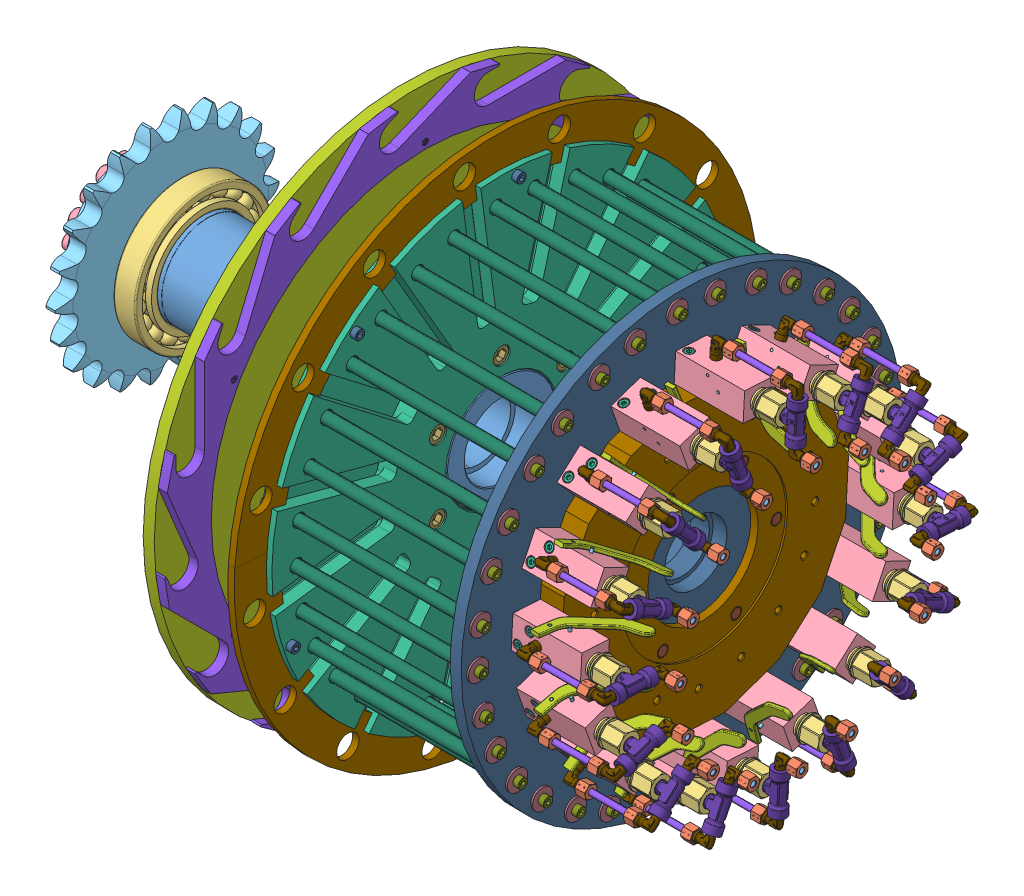
SolidWorks assembly Assieme1, configuration Default. Lengths in mm.
Overall size (749.63 778.63 778.63).
555 component instances, 28 part files, 75 mates.
Components (placement in the parent):
- albero rotazione piatti-1: albero rotazione piatti [Default] at (60.413 18.3637 415) size (415 200 200)
- seger 100mm-1: seger 100mm [KS 1336 E - 100] at (-146.4567 18.3637 415) x (0 0 -1) z (1 0 0) size (107.55 112.98 3)
- SKF - 6020 - 20,DE,NC,20_68-1: SKF - 6020 - 20,DE,NC,20_68 [SKF - 6020 - 20,DE,NC,20_68] at (-131.4567 18.3637 415) x (1 0 0) z (0 -0.434476 -0.900684) size (24 150 150)
- calettatore d95-1: calettatore d95 [Default] at (-184.9572 18.3637 415) size (39.5 135 135)
- pulegia z =50-1: pulegia z =50 [Chain wheel ISO - 22Z 20A-1 --22SB150H40L95.0N] at (-173.9167 18.3637 415) size (40 241.57 243.73)
- Disco supporto montaggio e Colonne-1: Disco supporto montaggio e Colonne [Default] at (204.0433 18.3637 415) x (0 -0.866025 -0.5) z (1 0 0) size (499.6 499.6 29)
- SKF - 6020 - 20,DE,NC,20_68-2: SKF - 6020 - 20,DE,NC,20_68 [SKF - 6020 - 20,DE,NC,20_68] at (62.0433 18.3637 415) x (1 0 0) z (0 -0.432628 -0.901573) size (24 150 150)
- piatto rotante porta tappi-1: piatto rotante porta tappi [Default] at (99.0433 18.3637 415) x (0 0 -1) z (1 0 0) size (570 570 20.57)
- disco trasportatore tappi 31-1: disco trasportatore tappi 31 [Default] at (111.0433 18.3637 415) x (0 0.5 -0.866025) z (1 0 0) size (570 570 10.42)
- Distributore Rotante-1: Distributore Rotante [Default] at (425.0433 18.3637 415) x (0 -0.055301 -0.99847) z (1 0 0) size (310 310 25.54)
- disco trascinato porta distributore vuoto-1: disco trascinato porta distributore vuoto [Default] at (400.0433 18.3637 415) x (0 0.055301 0.99847) z (-1 0 0) size (480 480 50)
- m12 35mm-1: m12 35mm [ISO 4762 M12 x 35 - 35N] at (376.0433 -53.0243 378.8925) x (1 0 0) z (0 -0.5 0.866025) size (47 18 18)
- m12 90mm-3: m12 90mm [ISO 4762 M12 x 90 - 90N] at (203.0433 -21.6363 345.718) x (-1 0 0) z (0 -0.5 0.866025) size (102 18 18)
- rondella m6 22mm-1: rondella m6 22mm [Washer ISO 7094 - 6] at (99.0433 -101.6363 207.1539) x (1 0 0) z (0 -1 0) size (2 22 22)
- M6 20mm-1: M6 20mm [ISO 4762 M6 x 20 - 20N] at (91.0433 -101.6363 207.1539) x (1 0 0) z (0 0.5 0.866025) size (26 10 10)
- m12 35mm-2: m12 35mm [ISO 4762 M12 x 35 - 35N] at (376.0433 13.9397 335.1224) x (1 0 0) z (0 -1 0) size (47 18 18)
- m12 35mm-3: m12 35mm [ISO 4762 M12 x 35 - 35N] at (376.0433 85.3277 371.2299) x (1 0 0) z (0 -0.5 -0.866025) size (47 18 18)
- m12 35mm-4: m12 35mm [ISO 4762 M12 x 35 - 35N] at (376.0433 89.7517 451.1075) x (1 0 0) z (0 0.5 -0.866025) size (47 18 18)
- m12 35mm-5: m12 35mm [ISO 4762 M12 x 35 - 35N] at (376.0433 22.7877 494.8776) x (1 0 0) z (0 1 0) size (47 18 18)
- m12 35mm-6: m12 35mm [ISO 4762 M12 x 35 - 35N] at (376.0433 -48.6003 458.7701) x (1 0 0) z (0 0.5 0.866025) size (47 18 18)
- rondella m6 22mm-2: rondella m6 22mm [Washer ISO 7094 - 6] at (99.0433 138.3637 207.1539) x (1 0 0) z (0 -0.5 -0.866025) size (2 22 22)
- rondella m6 22mm-3: rondella m6 22mm [Washer ISO 7094 - 6] at (99.0433 258.3637 415) x (1 0 0) z (0 0.5 -0.866025) size (2 22 22)
- rondella m6 22mm-4: rondella m6 22mm [Washer ISO 7094 - 6] at (99.0433 138.3637 622.8461) x (1 0 0) z (0 1 0) size (2 22 22)
- rondella m6 22mm-5: rondella m6 22mm [Washer ISO 7094 - 6] at (99.0433 -101.6363 622.8461) x (1 0 0) z (0 0.5 0.866025) size (2 22 22)
- rondella m6 22mm-6: rondella m6 22mm [Washer ISO 7094 - 6] at (99.0433 -221.6363 415) x (1 0 0) z (0 -0.5 0.866025) size (2 22 22)
- M6 20mm-2: M6 20mm [ISO 4762 M6 x 20 - 20N] at (91.0433 138.3637 207.1539) x (1 0 0) z (0 -0.5 0.866025) size (26 10 10)
- M6 20mm-3: M6 20mm [ISO 4762 M6 x 20 - 20N] at (91.0433 258.3637 415) x (1 0 0) z (0 -1 0) size (26 10 10)
- M6 20mm-4: M6 20mm [ISO 4762 M6 x 20 - 20N] at (91.0433 138.3637 622.8461) x (1 0 0) z (0 -0.5 -0.866025) size (26 10 10)
- M6 20mm-5: M6 20mm [ISO 4762 M6 x 20 - 20N] at (91.0433 -101.6363 622.8461) x (1 0 0) z (0 0.5 -0.866025) size (26 10 10)
- M6 20mm-6: M6 20mm [ISO 4762 M6 x 20 - 20N] at (91.0433 -221.6363 415) x (1 0 0) z (0 1 0) size (26 10 10)
- m12 90mm-4: m12 90mm [ISO 4762 M12 x 90 - 90N] at (203.0433 58.3637 345.718) x (-1 0 0) z (0 -1 0) size (102 18 18)
- m12 90mm-5: m12 90mm [ISO 4762 M12 x 90 - 90N] at (203.0433 98.3637 415) x (-1 0 0) z (0 -0.5 -0.866025) size (102 18 18)
- m12 90mm-6: m12 90mm [ISO 4762 M12 x 90 - 90N] at (203.0433 58.3637 484.282) x (-1 0 0) z (0 0.5 -0.866025) size (102 18 18)
- m12 90mm-7: m12 90mm [ISO 4762 M12 x 90 - 90N] at (203.0433 -21.6363 484.282) x (-1 0 0) z (0 1 0) size (102 18 18)
- m12 90mm-8: m12 90mm [ISO 4762 M12 x 90 - 90N] at (203.0433 -61.6363 415) x (-1 0 0) z (0 0.5 0.866025) size (102 18 18)
- asta scorrimento carello-1: asta scorrimento carello [Default] at (287.5433 70.1437 197.9013) x (0 0 -1) z (1 0 0) size (12 12 225)
- rondella m6 22mm-7: rondella m6 22mm [Washer ISO 7094 - 6] at (175.0433 70.1437 197.9013) x (1 0 0) z (0 -1 0) size (2 22 22)
- M6 16mm-1: M6 16mm [ISO 4762 M6 x 16 - 16N] at (167.0433 70.1437 197.9013) size (22 10 10)
- M6 16mm-2: M6 16mm [ISO 4762 M6 x 16 - 16N] at (408.0433 70.1437 197.9013) x (-1 0 0) z (0 0 -1) size (22 10 10)
- rondella m6 22mm-8: rondella m6 22mm [Washer ISO 7094 - 6] at (400.0433 70.1437 197.9013) x (-1 0 0) z (0 1 0) size (2 22 22)
- rondella m6 22mm-9: rondella m6 22mm [Washer ISO 7094 - 6] at (175.0433 24.5373 191.8971) x (1 0 0) z (0 -0.965926 -0.258819) size (2 22 22)
- M6 16mm-3: M6 16mm [ISO 4762 M6 x 16 - 16N] at (167.0433 24.5373 191.8971) x (1 0 0) z (0 0.258819 -0.965926) size (22 10 10)
- asta scorrimento carello-2: asta scorrimento carello [Default] at (287.5433 24.5373 191.8971) x (0 0.258819 -0.965926) z (-1 0 0) size (12 12 225)
- rondella m6 22mm-10: rondella m6 22mm [Washer ISO 7094 - 6] at (400.0433 24.5373 191.8971) x (-1 0 0) z (0 0.965926 0.258819) size (2 22 22)
- M6 16mm-4: M6 16mm [ISO 4762 M6 x 16 - 16N] at (408.0433 24.5373 191.8971) x (-1 0 0) z (0 -0.258819 0.965926) size (22 10 10)
- AssiemeValvola-1: AssiemeValvola [Default] at (515.3257 74.6348 254.5832) x (0 -0.331007 0.943628) z (0 0.943628 0.331007) size (90.26 138.63 38)
  - RaccordoT-1: RaccordoT [Default] at origin size (43 29.75 16.5)
  - Raccordo a L-1: Raccordo a L [Default] at (-30 0 0) x (0 -1 0) z (0 0 -1) size (28.34 25.51 14.01)
    - 1809_06_10_01-1: 1809_06_10_01 [Default] at origin size (22.49 23 10)
    - 1809_06_10_02-1: 1809_06_10_02 [Default] at origin size (6.5 8.5 8.5)
    - 1809_06_10_03-1: 1809_06_10_03 [Default] at origin size (11.02 15.01 14.01)
  - Raccordo a L-2: Raccordo a L [Default] at (30 0 0) x (0 1 0) z (0 0 -1) size (28.34 25.51 14.01)
    - 1809_06_10_01-1: 1809_06_10_01 [Default] at origin size (22.49 23 10)
    - 1809_06_10_02-1: 1809_06_10_02 [Default] at origin size (6.5 8.5 8.5)
    - 1809_06_10_03-1: 1809_06_10_03 [Default] at origin size (11.02 15.01 14.01)
  - TappoChiusura-1: TappoChiusura [Default] at (0 -32 0) x (0 -1 0) z (0 0 1) size (38.28 26.74 26.74)
  - CorpoValvola-1: CorpoValvola [Default] at (-15 -115.2824 0) size (30 75 34)
  - Raccordo a L-3: Raccordo a L [Default] at (-30 -88.2824 0) x (0 1 0) z (0 0 1) size (28.34 25.51 14.01)
    - 1809_06_10_01-1: 1809_06_10_01 [Default] at origin size (22.49 23 10)
    - 1809_06_10_02-1: 1809_06_10_02 [Default] at origin size (6.5 8.5 8.5)
    - 1809_06_10_03-1: 1809_06_10_03 [Default] at origin size (11.02 15.01 14.01)
  - Spina_3x38-1: Spina_3x38 [Default] at (0 -68.2824 -21) x (-1 0 0) z (0 0 1) size (3 3 38)
  - Spina_3x38-2: Spina_3x38 [Default] at (-10 -80.2824 -21) x (0.996193 0.087174 0) z (0 0 1) size (3 3 38)
  - M5 40mm-3: M5 40mm [ISO 4762 M5 x 40 - 40N] at (-14.6 -108.7824 9) size (45 8.5 8.5)
  - M5 40mm-2: M5 40mm [ISO 4762 M5 x 40 - 40N] at (-14.6 -96.7824 -9) size (45 8.5 8.5)
  - LevaValvola-1: LevaValvola [Default] at (-24.507 -86.571 -17) x (0.996193 0.087174 0) z (0 0 1) size (77.55 60.2 4)
  - Tubo-1: Tubo [Default] at (-30 -15.9665 0) x (1 0 0) z (0 -1 0) size (6 6 56.4)
- M6 16mm-5: M6 16mm [ISO 4762 M6 x 16 - 16N] at (167.0433 -16.8778 194.6116) x (1 0 0) z (0 0.382683 0.92388) size (22 10 10)
- M6 16mm-6: M6 16mm [ISO 4762 M6 x 16 - 16N] at (167.0433 -98.5342 224.874) x (1 0 0) z (0 0.707107 0.707107) size (22 10 10)
- M6 16mm-7: M6 16mm [ISO 4762 M6 x 16 - 16N] at (167.0433 -162.3939 284.0814) x (1 0 0) z (0 0.92388 0.382683) size (22 10 10)
- M6 16mm-8: M6 16mm [ISO 4762 M6 x 16 - 16N] at (167.0433 -198.735 363.22) x (1 0 0) z (0 1 0) size (22 10 10)
- M6 16mm-9: M6 16mm [ISO 4762 M6 x 16 - 16N] at (167.0433 -202.0247 450.2415) x (1 0 0) z (0 0.92388 -0.382683) size (22 10 10)
- M6 16mm-10: M6 16mm [ISO 4762 M6 x 16 - 16N] at (167.0433 -171.7623 531.8979) x (1 0 0) z (0 0.707107 -0.707107) size (22 10 10)
- M6 16mm-11: M6 16mm [ISO 4762 M6 x 16 - 16N] at (167.0433 -112.5549 595.7576) x (1 0 0) z (0 0.382683 -0.92388) size (22 10 10)
- M6 16mm-12: M6 16mm [ISO 4762 M6 x 16 - 16N] at (167.0433 -33.4163 632.0987) x (1 0 0) z (0 0 -1) size (22 10 10)
- M6 16mm-13: M6 16mm [ISO 4762 M6 x 16 - 16N] at (167.0433 53.6052 635.3884) x (1 0 0) z (0 -0.382683 -0.92388) size (22 10 10)
- M6 16mm-14: M6 16mm [ISO 4762 M6 x 16 - 16N] at (167.0433 135.2616 605.126) x (1 0 0) z (0 -0.707107 -0.707107) size (22 10 10)
- M6 16mm-15: M6 16mm [ISO 4762 M6 x 16 - 16N] at (167.0433 199.1213 545.9186) x (1 0 0) z (0 -0.92388 -0.382683) size (22 10 10)
- M6 16mm-16: M6 16mm [ISO 4762 M6 x 16 - 16N] at (167.0433 235.4624 466.78) x (1 0 0) z (0 -1 0) size (22 10 10)
- M6 16mm-17: M6 16mm [ISO 4762 M6 x 16 - 16N] at (167.0433 238.7521 379.7585) x (1 0 0) z (0 -0.92388 0.382683) size (22 10 10)
- M6 16mm-18: M6 16mm [ISO 4762 M6 x 16 - 16N] at (167.0433 208.4897 298.1021) x (1 0 0) z (0 -0.707107 0.707107) size (22 10 10)
- M6 16mm-19: M6 16mm [ISO 4762 M6 x 16 - 16N] at (167.0433 149.2823 234.2424) x (1 0 0) z (0 -0.382683 0.92388) size (22 10 10)
- rondella m6 22mm-11: rondella m6 22mm [Washer ISO 7094 - 6] at (175.0433 -16.8778 194.6116) x (1 0 0) z (0 -0.92388 0.382683) size (2 22 22)
- rondella m6 22mm-12: rondella m6 22mm [Washer ISO 7094 - 6] at (175.0433 -98.5342 224.874) x (1 0 0) z (0 -0.707107 0.707107) size (2 22 22)
- rondella m6 22mm-13: rondella m6 22mm [Washer ISO 7094 - 6] at (175.0433 -162.3939 284.0814) x (1 0 0) z (0 -0.382683 0.92388) size (2 22 22)
- rondella m6 22mm-14: rondella m6 22mm [Washer ISO 7094 - 6] at (175.0433 -198.735 363.22) size (2 22 22)
- rondella m6 22mm-15: rondella m6 22mm [Washer ISO 7094 - 6] at (175.0433 -202.0247 450.2415) x (1 0 0) z (0 0.382683 0.92388) size (2 22 22)
- rondella m6 22mm-16: rondella m6 22mm [Washer ISO 7094 - 6] at (175.0433 -171.7623 531.8979) x (1 0 0) z (0 0.707107 0.707107) size (2 22 22)
- rondella m6 22mm-17: rondella m6 22mm [Washer ISO 7094 - 6] at (175.0433 -112.5549 595.7576) x (1 0 0) z (0 0.92388 0.382683) size (2 22 22)
- rondella m6 22mm-18: rondella m6 22mm [Washer ISO 7094 - 6] at (175.0433 -33.4163 632.0987) x (1 0 0) z (0 1 0) size (2 22 22)
- rondella m6 22mm-19: rondella m6 22mm [Washer ISO 7094 - 6] at (175.0433 53.6052 635.3884) x (1 0 0) z (0 0.92388 -0.382683) size (2 22 22)
- rondella m6 22mm-20: rondella m6 22mm [Washer ISO 7094 - 6] at (175.0433 135.2616 605.126) x (1 0 0) z (0 0.707107 -0.707107) size (2 22 22)
- rondella m6 22mm-21: rondella m6 22mm [Washer ISO 7094 - 6] at (175.0433 199.1213 545.9186) x (1 0 0) z (0 0.382683 -0.92388) size (2 22 22)
- rondella m6 22mm-22: rondella m6 22mm [Washer ISO 7094 - 6] at (175.0433 235.4624 466.78) x (1 0 0) z (0 0 -1) size (2 22 22)
- rondella m6 22mm-23: rondella m6 22mm [Washer ISO 7094 - 6] at (175.0433 238.7521 379.7585) x (1 0 0) z (0 -0.382683 -0.92388) size (2 22 22)
- rondella m6 22mm-24: rondella m6 22mm [Washer ISO 7094 - 6] at (175.0433 208.4897 298.1021) x (1 0 0) z (0 -0.707107 -0.707107) size (2 22 22)
- rondella m6 22mm-25: rondella m6 22mm [Washer ISO 7094 - 6] at (175.0433 149.2823 234.2424) x (1 0 0) z (0 -0.92388 -0.382683) size (2 22 22)
- asta scorrimento carello-3: asta scorrimento carello [Default] at (287.5433 -16.8778 194.6116) x (0 -0.382683 -0.92388) z (1 0 0) size (12 12 225)
- asta scorrimento carello-4: asta scorrimento carello [Default] at (287.5433 -98.5342 224.874) x (0 -0.707107 -0.707107) z (1 0 0) size (12 12 225)
- asta scorrimento carello-5: asta scorrimento carello [Default] at (287.5433 -162.3939 284.0814) x (0 -0.92388 -0.382683) z (1 0 0) size (12 12 225)
- asta scorrimento carello-6: asta scorrimento carello [Default] at (287.5433 -198.735 363.22) x (0 -1 0) z (1 0 0) size (12 12 225)
- asta scorrimento carello-7: asta scorrimento carello [Default] at (287.5433 -202.0247 450.2415) x (0 -0.92388 0.382683) z (1 0 0) size (12 12 225)
- asta scorrimento carello-8: asta scorrimento carello [Default] at (287.5433 -171.7623 531.8979) x (0 -0.707107 0.707107) z (1 0 0) size (12 12 225)
- asta scorrimento carello-9: asta scorrimento carello [Default] at (287.5433 -112.5549 595.7576) x (0 -0.382683 0.92388) z (1 0 0) size (12 12 225)
- asta scorrimento carello-10: asta scorrimento carello [Default] at (287.5433 -33.4163 632.0987) x (0 0 1) z (1 0 0) size (12 12 225)
- asta scorrimento carello-11: asta scorrimento carello [Default] at (287.5433 53.6052 635.3884) x (0 0.382683 0.92388) z (1 0 0) size (12 12 225)
- asta scorrimento carello-12: asta scorrimento carello [Default] at (287.5433 135.2616 605.126) x (0 0.707107 0.707107) z (1 0 0) size (12 12 225)
- asta scorrimento carello-13: asta scorrimento carello [Default] at (287.5433 199.1213 545.9186) x (0 0.92388 0.382683) z (1 0 0) size (12 12 225)
- asta scorrimento carello-14: asta scorrimento carello [Default] at (287.5433 235.4624 466.78) x (0 1 0) z (1 0 0) size (12 12 225)
- asta scorrimento carello-15: asta scorrimento carello [Default] at (287.5433 238.7521 379.7585) x (0 0.92388 -0.382683) z (1 0 0) size (12 12 225)
- asta scorrimento carello-16: asta scorrimento carello [Default] at (287.5433 208.4897 298.1021) x (0 0.707107 -0.707107) z (1 0 0) size (12 12 225)
- asta scorrimento carello-17: asta scorrimento carello [Default] at (287.5433 149.2823 234.2424) x (0 0.382683 -0.92388) z (1 0 0) size (12 12 225)
- M6 16mm-20: M6 16mm [ISO 4762 M6 x 16 - 16N] at (408.0433 -16.8778 194.6116) x (-1 0 0) z (0 -0.382683 -0.92388) size (22 10 10)
- M6 16mm-21: M6 16mm [ISO 4762 M6 x 16 - 16N] at (408.0433 -98.5342 224.874) x (-1 0 0) z (0 -0.707107 -0.707107) size (22 10 10)
- M6 16mm-22: M6 16mm [ISO 4762 M6 x 16 - 16N] at (408.0433 -162.3939 284.0814) x (-1 0 0) z (0 -0.92388 -0.382683) size (22 10 10)
- M6 16mm-23: M6 16mm [ISO 4762 M6 x 16 - 16N] at (408.0433 -198.735 363.22) x (-1 0 0) z (0 -1 0) size (22 10 10)
- M6 16mm-24: M6 16mm [ISO 4762 M6 x 16 - 16N] at (408.0433 -202.0247 450.2415) x (-1 0 0) z (0 -0.92388 0.382683) size (22 10 10)
- M6 16mm-25: M6 16mm [ISO 4762 M6 x 16 - 16N] at (408.0433 -171.7623 531.8979) x (-1 0 0) z (0 -0.707107 0.707107) size (22 10 10)
- M6 16mm-26: M6 16mm [ISO 4762 M6 x 16 - 16N] at (408.0433 -112.5549 595.7576) x (-1 0 0) z (0 -0.382683 0.92388) size (22 10 10)
- M6 16mm-27: M6 16mm [ISO 4762 M6 x 16 - 16N] at (408.0433 -33.4163 632.0987) x (-1 0 0) z (0 0 1) size (22 10 10)
- M6 16mm-28: M6 16mm [ISO 4762 M6 x 16 - 16N] at (408.0433 53.6052 635.3884) x (-1 0 0) z (0 0.382683 0.92388) size (22 10 10)
- M6 16mm-29: M6 16mm [ISO 4762 M6 x 16 - 16N] at (408.0433 135.2616 605.126) x (-1 0 0) z (0 0.707107 0.707107) size (22 10 10)
- M6 16mm-30: M6 16mm [ISO 4762 M6 x 16 - 16N] at (408.0433 199.1213 545.9186) x (-1 0 0) z (0 0.92388 0.382683) size (22 10 10)
- M6 16mm-31: M6 16mm [ISO 4762 M6 x 16 - 16N] at (408.0433 235.4624 466.78) x (-1 0 0) z (0 1 0) size (22 10 10)
- M6 16mm-32: M6 16mm [ISO 4762 M6 x 16 - 16N] at (408.0433 238.7521 379.7585) x (-1 0 0) z (0 0.92388 -0.382683) size (22 10 10)
- M6 16mm-33: M6 16mm [ISO 4762 M6 x 16 - 16N] at (408.0433 208.4897 298.1021) x (-1 0 0) z (0 0.707107 -0.707107) size (22 10 10)
- M6 16mm-34: M6 16mm [ISO 4762 M6 x 16 - 16N] at (408.0433 149.2823 234.2424) x (-1 0 0) z (0 0.382683 -0.92388) size (22 10 10)
- rondella m6 22mm-26: rondella m6 22mm [Washer ISO 7094 - 6] at (400.0433 -16.8778 194.6116) x (-1 0 0) z (0 0.92388 -0.382683) size (2 22 22)
- rondella m6 22mm-27: rondella m6 22mm [Washer ISO 7094 - 6] at (400.0433 -98.5342 224.874) x (-1 0 0) z (0 0.707107 -0.707107) size (2 22 22)
- rondella m6 22mm-28: rondella m6 22mm [Washer ISO 7094 - 6] at (400.0433 -162.3939 284.0814) x (-1 0 0) z (0 0.382683 -0.92388) size (2 22 22)
- rondella m6 22mm-29: rondella m6 22mm [Washer ISO 7094 - 6] at (400.0433 -198.735 363.22) x (-1 0 0) z (0 0 -1) size (2 22 22)
- rondella m6 22mm-30: rondella m6 22mm [Washer ISO 7094 - 6] at (400.0433 -202.0247 450.2415) x (-1 0 0) z (0 -0.382683 -0.92388) size (2 22 22)
- rondella m6 22mm-31: rondella m6 22mm [Washer ISO 7094 - 6] at (400.0433 -171.7623 531.8979) x (-1 0 0) z (0 -0.707107 -0.707107) size (2 22 22)
- rondella m6 22mm-32: rondella m6 22mm [Washer ISO 7094 - 6] at (400.0433 -112.5549 595.7576) x (-1 0 0) z (0 -0.92388 -0.382683) size (2 22 22)
- rondella m6 22mm-33: rondella m6 22mm [Washer ISO 7094 - 6] at (400.0433 -33.4163 632.0987) x (-1 0 0) z (0 -1 0) size (2 22 22)
- rondella m6 22mm-34: rondella m6 22mm [Washer ISO 7094 - 6] at (400.0433 53.6052 635.3884) x (-1 0 0) z (0 -0.92388 0.382683) size (2 22 22)
- rondella m6 22mm-35: rondella m6 22mm [Washer ISO 7094 - 6] at (400.0433 135.2616 605.126) x (-1 0 0) z (0 -0.707107 0.707107) size (2 22 22)
- rondella m6 22mm-36: rondella m6 22mm [Washer ISO 7094 - 6] at (400.0433 199.1213 545.9186) x (-1 0 0) z (0 -0.382683 0.92388) size (2 22 22)
- rondella m6 22mm-37: rondella m6 22mm [Washer ISO 7094 - 6] at (400.0433 235.4624 466.78) x (-1 0 0) z (0 0 1) size (2 22 22)
- rondella m6 22mm-38: rondella m6 22mm [Washer ISO 7094 - 6] at (400.0433 238.7521 379.7585) x (-1 0 0) z (0 0.382683 0.92388) size (2 22 22)
- rondella m6 22mm-39: rondella m6 22mm [Washer ISO 7094 - 6] at (400.0433 208.4897 298.1021) x (-1 0 0) z (0 0.707107 0.707107) size (2 22 22)
- rondella m6 22mm-40: rondella m6 22mm [Washer ISO 7094 - 6] at (400.0433 149.2823 234.2424) x (-1 0 0) z (0 0.92388 0.382683) size (2 22 22)
- rondella m6 22mm-41: rondella m6 22mm [Washer ISO 7094 - 6] at (175.0433 -61.3104 206.5173) x (1 0 0) z (0 -0.991445 0.130526) size (2 22 22)
- rondella m6 22mm-42: rondella m6 22mm [Washer ISO 7094 - 6] at (175.0433 -135.0285 252.8771) x (1 0 0) z (0 -0.866025 0.5) size (2 22 22)
- rondella m6 22mm-43: rondella m6 22mm [Washer ISO 7094 - 6] at (175.0433 -185.3939 323.9186) x (1 0 0) z (0 -0.608761 0.793353) size (2 22 22)
- rondella m6 22mm-44: rondella m6 22mm [Washer ISO 7094 - 6] at (175.0433 -204.7392 408.8264) x (1 0 0) z (0 -0.258819 0.965926) size (2 22 22)
- rondella m6 22mm-45: rondella m6 22mm [Washer ISO 7094 - 6] at (175.0433 -190.119 494.6741) x (1 0 0) z (0 0.130526 0.991445) size (2 22 22)
- rondella m6 22mm-46: rondella m6 22mm [Washer ISO 7094 - 6] at (175.0433 -143.7592 568.3922) x (1 0 0) z (0 0.5 0.866025) size (2 22 22)
- rondella m6 22mm-47: rondella m6 22mm [Washer ISO 7094 - 6] at (175.0433 -72.7177 618.7576) x (1 0 0) z (0 0.793353 0.608761) size (2 22 22)
- rondella m6 22mm-48: rondella m6 22mm [Washer ISO 7094 - 6] at (175.0433 12.1901 638.1029) x (1 0 0) z (0 0.965926 0.258819) size (2 22 22)
- rondella m6 22mm-49: rondella m6 22mm [Washer ISO 7094 - 6] at (175.0433 98.0378 623.4827) x (1 0 0) z (0 0.991445 -0.130526) size (2 22 22)
- rondella m6 22mm-50: rondella m6 22mm [Washer ISO 7094 - 6] at (175.0433 171.7559 577.1229) x (1 0 0) z (0 0.866025 -0.5) size (2 22 22)
- rondella m6 22mm-51: rondella m6 22mm [Washer ISO 7094 - 6] at (175.0433 222.1213 506.0814) x (1 0 0) z (0 0.608761 -0.793353) size (2 22 22)
- rondella m6 22mm-52: rondella m6 22mm [Washer ISO 7094 - 6] at (175.0433 241.4666 421.1736) x (1 0 0) z (0 0.258819 -0.965926) size (2 22 22)
- rondella m6 22mm-53: rondella m6 22mm [Washer ISO 7094 - 6] at (175.0433 226.8464 335.3259) x (1 0 0) z (0 -0.130526 -0.991445) size (2 22 22)
- rondella m6 22mm-54: rondella m6 22mm [Washer ISO 7094 - 6] at (175.0433 180.4866 261.6078) x (1 0 0) z (0 -0.5 -0.866025) size (2 22 22)
- rondella m6 22mm-55: rondella m6 22mm [Washer ISO 7094 - 6] at (175.0433 109.4451 211.2424) x (1 0 0) z (0 -0.793353 -0.608761) size (2 22 22)
- M6 16mm-35: M6 16mm [ISO 4762 M6 x 16 - 16N] at (167.0433 -61.3104 206.5173) x (1 0 0) z (0 -0.130526 -0.991445) size (22 10 10)
- M6 16mm-36: M6 16mm [ISO 4762 M6 x 16 - 16N] at (167.0433 -135.0285 252.8771) x (1 0 0) z (0 -0.5 -0.866025) size (22 10 10)
- M6 16mm-37: M6 16mm [ISO 4762 M6 x 16 - 16N] at (167.0433 -185.3939 323.9186) x (1 0 0) z (0 -0.793353 -0.608761) size (22 10 10)
- M6 16mm-38: M6 16mm [ISO 4762 M6 x 16 - 16N] at (167.0433 -204.7392 408.8264) x (1 0 0) z (0 -0.965926 -0.258819) size (22 10 10)
- M6 16mm-39: M6 16mm [ISO 4762 M6 x 16 - 16N] at (167.0433 -190.119 494.6741) x (1 0 0) z (0 -0.991445 0.130526) size (22 10 10)
- M6 16mm-40: M6 16mm [ISO 4762 M6 x 16 - 16N] at (167.0433 -143.7592 568.3922) x (1 0 0) z (0 -0.866025 0.5) size (22 10 10)
- M6 16mm-41: M6 16mm [ISO 4762 M6 x 16 - 16N] at (167.0433 -72.7177 618.7576) x (1 0 0) z (0 -0.608761 0.793353) size (22 10 10)
- M6 16mm-42: M6 16mm [ISO 4762 M6 x 16 - 16N] at (167.0433 12.1901 638.1029) x (1 0 0) z (0 -0.258819 0.965926) size (22 10 10)
- M6 16mm-43: M6 16mm [ISO 4762 M6 x 16 - 16N] at (167.0433 98.0378 623.4827) x (1 0 0) z (0 0.130526 0.991445) size (22 10 10)
- M6 16mm-44: M6 16mm [ISO 4762 M6 x 16 - 16N] at (167.0433 171.7559 577.1229) x (1 0 0) z (0 0.5 0.866025) size (22 10 10)
- M6 16mm-45: M6 16mm [ISO 4762 M6 x 16 - 16N] at (167.0433 222.1213 506.0814) x (1 0 0) z (0 0.793353 0.608761) size (22 10 10)
- M6 16mm-46: M6 16mm [ISO 4762 M6 x 16 - 16N] at (167.0433 241.4666 421.1736) x (1 0 0) z (0 0.965926 0.258819) size (22 10 10)
- M6 16mm-47: M6 16mm [ISO 4762 M6 x 16 - 16N] at (167.0433 226.8464 335.3259) x (1 0 0) z (0 0.991445 -0.130526) size (22 10 10)
- M6 16mm-48: M6 16mm [ISO 4762 M6 x 16 - 16N] at (167.0433 180.4866 261.6078) x (1 0 0) z (0 0.866025 -0.5) size (22 10 10)
- M6 16mm-49: M6 16mm [ISO 4762 M6 x 16 - 16N] at (167.0433 109.4451 211.2424) x (1 0 0) z (0 0.608761 -0.793353) size (22 10 10)
- asta scorrimento carello-18: asta scorrimento carello [Default] at (287.5433 -61.3104 206.5173) x (0 -0.130526 -0.991445) z (-1 0 0) size (12 12 225)
- asta scorrimento carello-19: asta scorrimento carello [Default] at (287.5433 -135.0285 252.8771) x (0 -0.5 -0.866025) z (-1 0 0) size (12 12 225)
- asta scorrimento carello-20: asta scorrimento carello [Default] at (287.5433 -185.3939 323.9186) x (0 -0.793353 -0.608761) z (-1 0 0) size (12 12 225)
- asta scorrimento carello-21: asta scorrimento carello [Default] at (287.5433 -204.7392 408.8264) x (0 -0.965926 -0.258819) z (-1 0 0) size (12 12 225)
- asta scorrimento carello-22: asta scorrimento carello [Default] at (287.5433 -190.119 494.6741) x (0 -0.991445 0.130526) z (-1 0 0) size (12 12 225)
- asta scorrimento carello-23: asta scorrimento carello [Default] at (287.5433 -143.7592 568.3922) x (0 -0.866025 0.5) z (-1 0 0) size (12 12 225)
- asta scorrimento carello-24: asta scorrimento carello [Default] at (287.5433 -72.7177 618.7576) x (0 -0.608761 0.793353) z (-1 0 0) size (12 12 225)
- asta scorrimento carello-25: asta scorrimento carello [Default] at (287.5433 12.1901 638.1029) x (0 -0.258819 0.965926) z (-1 0 0) size (12 12 225)
- asta scorrimento carello-26: asta scorrimento carello [Default] at (287.5433 98.0378 623.4827) x (0 0.130526 0.991445) z (-1 0 0) size (12 12 225)
- asta scorrimento carello-27: asta scorrimento carello [Default] at (287.5433 171.7559 577.1229) x (0 0.5 0.866025) z (-1 0 0) size (12 12 225)
- asta scorrimento carello-28: asta scorrimento carello [Default] at (287.5433 222.1213 506.0814) x (0 0.793353 0.608761) z (-1 0 0) size (12 12 225)
- asta scorrimento carello-29: asta scorrimento carello [Default] at (287.5433 241.4666 421.1736) x (0 0.965926 0.258819) z (-1 0 0) size (12 12 225)
- asta scorrimento carello-30: asta scorrimento carello [Default] at (287.5433 226.8464 335.3259) x (0 0.991445 -0.130526) z (-1 0 0) size (12 12 225)
- asta scorrimento carello-31: asta scorrimento carello [Default] at (287.5433 180.4866 261.6078) x (0 0.866025 -0.5) z (-1 0 0) size (12 12 225)
- asta scorrimento carello-32: asta scorrimento carello [Default] at (287.5433 109.4451 211.2424) x (0 0.608761 -0.793353) z (-1 0 0) size (12 12 225)
- rondella m6 22mm-56: rondella m6 22mm [Washer ISO 7094 - 6] at (400.0433 -61.3104 206.5173) x (-1 0 0) z (0 0.991445 -0.130526) size (2 22 22)
- rondella m6 22mm-57: rondella m6 22mm [Washer ISO 7094 - 6] at (400.0433 -135.0285 252.8771) x (-1 0 0) z (0 0.866025 -0.5) size (2 22 22)
- rondella m6 22mm-58: rondella m6 22mm [Washer ISO 7094 - 6] at (400.0433 -185.3939 323.9186) x (-1 0 0) z (0 0.608761 -0.793353) size (2 22 22)
- rondella m6 22mm-59: rondella m6 22mm [Washer ISO 7094 - 6] at (400.0433 -204.7392 408.8264) x (-1 0 0) z (0 0.258819 -0.965926) size (2 22 22)
- rondella m6 22mm-60: rondella m6 22mm [Washer ISO 7094 - 6] at (400.0433 -190.119 494.6741) x (-1 0 0) z (0 -0.130526 -0.991445) size (2 22 22)
- rondella m6 22mm-61: rondella m6 22mm [Washer ISO 7094 - 6] at (400.0433 -143.7592 568.3922) x (-1 0 0) z (0 -0.5 -0.866025) size (2 22 22)
- rondella m6 22mm-62: rondella m6 22mm [Washer ISO 7094 - 6] at (400.0433 -72.7177 618.7576) x (-1 0 0) z (0 -0.793353 -0.608761) size (2 22 22)
- rondella m6 22mm-63: rondella m6 22mm [Washer ISO 7094 - 6] at (400.0433 12.1901 638.1029) x (-1 0 0) z (0 -0.965926 -0.258819) size (2 22 22)
- rondella m6 22mm-64: rondella m6 22mm [Washer ISO 7094 - 6] at (400.0433 98.0378 623.4827) x (-1 0 0) z (0 -0.991445 0.130526) size (2 22 22)
- rondella m6 22mm-65: rondella m6 22mm [Washer ISO 7094 - 6] at (400.0433 171.7559 577.1229) x (-1 0 0) z (0 -0.866025 0.5) size (2 22 22)
- rondella m6 22mm-66: rondella m6 22mm [Washer ISO 7094 - 6] at (400.0433 222.1213 506.0814) x (-1 0 0) z (0 -0.608761 0.793353) size (2 22 22)
- rondella m6 22mm-67: rondella m6 22mm [Washer ISO 7094 - 6] at (400.0433 241.4666 421.1736) x (-1 0 0) z (0 -0.258819 0.965926) size (2 22 22)
- rondella m6 22mm-68: rondella m6 22mm [Washer ISO 7094 - 6] at (400.0433 226.8464 335.3259) x (-1 0 0) z (0 0.130526 0.991445) size (2 22 22)
- rondella m6 22mm-69: rondella m6 22mm [Washer ISO 7094 - 6] at (400.0433 180.4866 261.6078) x (-1 0 0) z (0 0.5 0.866025) size (2 22 22)
- rondella m6 22mm-70: rondella m6 22mm [Washer ISO 7094 - 6] at (400.0433 109.4451 211.2424) x (-1 0 0) z (0 0.793353 0.608761) size (2 22 22)
- M6 16mm-50: M6 16mm [ISO 4762 M6 x 16 - 16N] at (408.0433 -61.3104 206.5173) x (-1 0 0) z (0 0.130526 0.991445) size (22 10 10)
- M6 16mm-51: M6 16mm [ISO 4762 M6 x 16 - 16N] at (408.0433 -135.0285 252.8771) x (-1 0 0) z (0 0.5 0.866025) size (22 10 10)
- M6 16mm-52: M6 16mm [ISO 4762 M6 x 16 - 16N] at (408.0433 -185.3939 323.9186) x (-1 0 0) z (0 0.793353 0.608761) size (22 10 10)
- M6 16mm-53: M6 16mm [ISO 4762 M6 x 16 - 16N] at (408.0433 -204.7392 408.8264) x (-1 0 0) z (0 0.965926 0.258819) size (22 10 10)
- M6 16mm-54: M6 16mm [ISO 4762 M6 x 16 - 16N] at (408.0433 -190.119 494.6741) x (-1 0 0) z (0 0.991445 -0.130526) size (22 10 10)
- M6 16mm-55: M6 16mm [ISO 4762 M6 x 16 - 16N] at (408.0433 -143.7592 568.3922) x (-1 0 0) z (0 0.866025 -0.5) size (22 10 10)
- M6 16mm-56: M6 16mm [ISO 4762 M6 x 16 - 16N] at (408.0433 -72.7177 618.7576) x (-1 0 0) z (0 0.608761 -0.793353) size (22 10 10)
- M6 16mm-57: M6 16mm [ISO 4762 M6 x 16 - 16N] at (408.0433 12.1901 638.1029) x (-1 0 0) z (0 0.258819 -0.965926) size (22 10 10)
- M6 16mm-58: M6 16mm [ISO 4762 M6 x 16 - 16N] at (408.0433 98.0378 623.4827) x (-1 0 0) z (0 -0.130526 -0.991445) size (22 10 10)
- M6 16mm-59: M6 16mm [ISO 4762 M6 x 16 - 16N] at (408.0433 171.7559 577.1229) x (-1 0 0) z (0 -0.5 -0.866025) size (22 10 10)
- M6 16mm-60: M6 16mm [ISO 4762 M6 x 16 - 16N] at (408.0433 222.1213 506.0814) x (-1 0 0) z (0 -0.793353 -0.608761) size (22 10 10)
- M6 16mm-61: M6 16mm [ISO 4762 M6 x 16 - 16N] at (408.0433 241.4666 421.1736) x (-1 0 0) z (0 -0.965926 -0.258819) size (22 10 10)
- M6 16mm-62: M6 16mm [ISO 4762 M6 x 16 - 16N] at (408.0433 226.8464 335.3259) x (-1 0 0) z (0 -0.991445 0.130526) size (22 10 10)
- M6 16mm-63: M6 16mm [ISO 4762 M6 x 16 - 16N] at (408.0433 180.4866 261.6078) x (-1 0 0) z (0 -0.866025 0.5) size (22 10 10)
- M6 16mm-64: M6 16mm [ISO 4762 M6 x 16 - 16N] at (408.0433 109.4451 211.2424) x (-1 0 0) z (0 -0.608761 0.793353) size (22 10 10)
- AssiemeValvola-2: AssiemeValvola [Default] at (515.3257 8.9626 245.2601) x (0 0.055301 0.99847) z (0 0.99847 -0.055301) size (90.26 138.63 38)
  - RaccordoT-1: RaccordoT [Default] at origin size (43 29.75 16.5)
  - Raccordo a L-1: Raccordo a L [Default] at (-30 0 0) x (0 -1 0) z (0 0 -1) size (28.34 25.51 14.01)
    - 1809_06_10_01-1: 1809_06_10_01 [Default] at origin size (22.49 23 10)
    - 1809_06_10_02-1: 1809_06_10_02 [Default] at origin size (6.5 8.5 8.5)
    - 1809_06_10_03-1: 1809_06_10_03 [Default] at origin size (11.02 15.01 14.01)
  - Raccordo a L-2: Raccordo a L [Default] at (30 0 0) x (0 1 0) z (0 0 -1) size (28.34 25.51 14.01)
    - 1809_06_10_01-1: 1809_06_10_01 [Default] at origin size (22.49 23 10)
    - 1809_06_10_02-1: 1809_06_10_02 [Default] at origin size (6.5 8.5 8.5)
    - 1809_06_10_03-1: 1809_06_10_03 [Default] at origin size (11.02 15.01 14.01)
  - TappoChiusura-1: TappoChiusura [Default] at (0 -32 0) x (0 -1 0) z (0 0 1) size (38.28 26.74 26.74)
  - CorpoValvola-1: CorpoValvola [Default] at (-15 -115.2824 0) size (30 75 34)
  - Raccordo a L-3: Raccordo a L [Default] at (-30 -88.2824 0) x (0 1 0) z (0 0 1) size (28.34 25.51 14.01)
    - 1809_06_10_01-1: 1809_06_10_01 [Default] at origin size (22.49 23 10)
    - 1809_06_10_02-1: 1809_06_10_02 [Default] at origin size (6.5 8.5 8.5)
    - 1809_06_10_03-1: 1809_06_10_03 [Default] at origin size (11.02 15.01 14.01)
  - Spina_3x38-1: Spina_3x38 [Default] at (0 -68.2824 -21) x (-1 0 0) z (0 0 1) size (3 3 38)
  - Spina_3x38-2: Spina_3x38 [Default] at (-10 -80.2824 -21) x (0.996193 0.087174 0) z (0 0 1) size (3 3 38)
  - M5 40mm-3: M5 40mm [ISO 4762 M5 x 40 - 40N] at (-14.6 -108.7824 9) size (45 8.5 8.5)
  - M5 40mm-2: M5 40mm [ISO 4762 M5 x 40 - 40N] at (-14.6 -96.7824 -9) size (45 8.5 8.5)
  - LevaValvola-1: LevaValvola [Default] at (-24.507 -86.571 -17) x (0.996193 0.087174 0) z (0 0 1) size (77.55 60.2 4)
  - Tubo-1: Tubo [Default] at (-30 -15.9665 0) x (1 0 0) z (0 -1 0) size (6 6 56.4)
- AssiemeValvola-3: AssiemeValvola [Default] at (515.3257 -55.2784 261.7785) x (0 0.433189 0.901303) z (0 0.901303 -0.433189) size (90.26 138.63 38)
  - RaccordoT-1: RaccordoT [Default] at origin size (43 29.75 16.5)
  - Raccordo a L-1: Raccordo a L [Default] at (-30 0 0) x (0 -1 0) z (0 0 -1) size (28.34 25.51 14.01)
    - 1809_06_10_01-1: 1809_06_10_01 [Default] at origin size (22.49 23 10)
    - 1809_06_10_02-1: 1809_06_10_02 [Default] at origin size (6.5 8.5 8.5)
    - 1809_06_10_03-1: 1809_06_10_03 [Default] at origin size (11.02 15.01 14.01)
  - Raccordo a L-2: Raccordo a L [Default] at (30 0 0) x (0 1 0) z (0 0 -1) size (28.34 25.51 14.01)
    - 1809_06_10_01-1: 1809_06_10_01 [Default] at origin size (22.49 23 10)
    - 1809_06_10_02-1: 1809_06_10_02 [Default] at origin size (6.5 8.5 8.5)
    - 1809_06_10_03-1: 1809_06_10_03 [Default] at origin size (11.02 15.01 14.01)
  - TappoChiusura-1: TappoChiusura [Default] at (0 -32 0) x (0 -1 0) z (0 0 1) size (38.28 26.74 26.74)
  - CorpoValvola-1: CorpoValvola [Default] at (-15 -115.2824 0) size (30 75 34)
  - Raccordo a L-3: Raccordo a L [Default] at (-30 -88.2824 0) x (0 1 0) z (0 0 1) size (28.34 25.51 14.01)
    - 1809_06_10_01-1: 1809_06_10_01 [Default] at origin size (22.49 23 10)
    - 1809_06_10_02-1: 1809_06_10_02 [Default] at origin size (6.5 8.5 8.5)
    - 1809_06_10_03-1: 1809_06_10_03 [Default] at origin size (11.02 15.01 14.01)
  - Spina_3x38-1: Spina_3x38 [Default] at (0 -68.2824 -21) x (-1 0 0) z (0 0 1) size (3 3 38)
  - Spina_3x38-2: Spina_3x38 [Default] at (-10 -80.2824 -21) x (0.996193 0.087174 0) z (0 0 1) size (3 3 38)
  - M5 40mm-3: M5 40mm [ISO 4762 M5 x 40 - 40N] at (-14.6 -108.7824 9) size (45 8.5 8.5)
  - M5 40mm-2: M5 40mm [ISO 4762 M5 x 40 - 40N] at (-14.6 -96.7824 -9) size (45 8.5 8.5)
  - LevaValvola-1: LevaValvola [Default] at (-24.507 -86.571 -17) x (0.996193 0.087174 0) z (0 0 1) size (77.55 60.2 4)
  - Tubo-1: Tubo [Default] at (-30 -15.9665 0) x (1 0 0) z (0 -1 0) size (6 6 56.4)
- AssiemeValvola-4: AssiemeValvola [Default] at (515.3257 -108.3081 301.6234) x (0 0.745128 0.666921) z (0 0.666921 -0.745128) size (90.26 138.63 38)
  - RaccordoT-1: RaccordoT [Default] at origin size (43 29.75 16.5)
  - Raccordo a L-1: Raccordo a L [Default] at (-30 0 0) x (0 -1 0) z (0 0 -1) size (28.34 25.51 14.01)
    - 1809_06_10_01-1: 1809_06_10_01 [Default] at origin size (22.49 23 10)
    - 1809_06_10_02-1: 1809_06_10_02 [Default] at origin size (6.5 8.5 8.5)
    - 1809_06_10_03-1: 1809_06_10_03 [Default] at origin size (11.02 15.01 14.01)
  - Raccordo a L-2: Raccordo a L [Default] at (30 0 0) x (0 1 0) z (0 0 -1) size (28.34 25.51 14.01)
    - 1809_06_10_01-1: 1809_06_10_01 [Default] at origin size (22.49 23 10)
    - 1809_06_10_02-1: 1809_06_10_02 [Default] at origin size (6.5 8.5 8.5)
    - 1809_06_10_03-1: 1809_06_10_03 [Default] at origin size (11.02 15.01 14.01)
  - TappoChiusura-1: TappoChiusura [Default] at (0 -32 0) x (0 -1 0) z (0 0 1) size (38.28 26.74 26.74)
  - CorpoValvola-1: CorpoValvola [Default] at (-15 -115.2824 0) size (30 75 34)
  - Raccordo a L-3: Raccordo a L [Default] at (-30 -88.2824 0) x (0 1 0) z (0 0 1) size (28.34 25.51 14.01)
    - 1809_06_10_01-1: 1809_06_10_01 [Default] at origin size (22.49 23 10)
    - 1809_06_10_02-1: 1809_06_10_02 [Default] at origin size (6.5 8.5 8.5)
    - 1809_06_10_03-1: 1809_06_10_03 [Default] at origin size (11.02 15.01 14.01)
  - Spina_3x38-1: Spina_3x38 [Default] at (0 -68.2824 -21) x (-1 0 0) z (0 0 1) size (3 3 38)
  - Spina_3x38-2: Spina_3x38 [Default] at (-10 -80.2824 -21) x (0.996193 0.087174 0) z (0 0 1) size (3 3 38)
  - M5 40mm-3: M5 40mm [ISO 4762 M5 x 40 - 40N] at (-14.6 -108.7824 9) size (45 8.5 8.5)
  - M5 40mm-2: M5 40mm [ISO 4762 M5 x 40 - 40N] at (-14.6 -96.7824 -9) size (45 8.5 8.5)
  - LevaValvola-1: LevaValvola [Default] at (-24.507 -86.571 -17) x (0.996193 0.087174 0) z (0 0 1) size (77.55 60.2 4)
  - Tubo-1: Tubo [Default] at (-30 -15.9665 0) x (1 0 0) z (0 -1 0) size (6 6 56.4)
- AssiemeValvola-5: AssiemeValvola [Default] at (515.3257 -142.0531 358.7289) x (0 0.943628 0.331007) z (0 0.331007 -0.943628) size (90.26 138.63 38)
  - RaccordoT-1: RaccordoT [Default] at origin size (43 29.75 16.5)
  - Raccordo a L-1: Raccordo a L [Default] at (-30 0 0) x (0 -1 0) z (0 0 -1) size (28.34 25.51 14.01)
    - 1809_06_10_01-1: 1809_06_10_01 [Default] at origin size (22.49 23 10)
    - 1809_06_10_02-1: 1809_06_10_02 [Default] at origin size (6.5 8.5 8.5)
    - 1809_06_10_03-1: 1809_06_10_03 [Default] at origin size (11.02 15.01 14.01)
  - Raccordo a L-2: Raccordo a L [Default] at (30 0 0) x (0 1 0) z (0 0 -1) size (28.34 25.51 14.01)
    - 1809_06_10_01-1: 1809_06_10_01 [Default] at origin size (22.49 23 10)
    - 1809_06_10_02-1: 1809_06_10_02 [Default] at origin size (6.5 8.5 8.5)
    - 1809_06_10_03-1: 1809_06_10_03 [Default] at origin size (11.02 15.01 14.01)
  - TappoChiusura-1: TappoChiusura [Default] at (0 -32 0) x (0 -1 0) z (0 0 1) size (38.28 26.74 26.74)
  - CorpoValvola-1: CorpoValvola [Default] at (-15 -115.2824 0) size (30 75 34)
  - Raccordo a L-3: Raccordo a L [Default] at (-30 -88.2824 0) x (0 1 0) z (0 0 1) size (28.34 25.51 14.01)
    - 1809_06_10_01-1: 1809_06_10_01 [Default] at origin size (22.49 23 10)
    - 1809_06_10_02-1: 1809_06_10_02 [Default] at origin size (6.5 8.5 8.5)
    - 1809_06_10_03-1: 1809_06_10_03 [Default] at origin size (11.02 15.01 14.01)
  - Spina_3x38-1: Spina_3x38 [Default] at (0 -68.2824 -21) x (-1 0 0) z (0 0 1) size (3 3 38)
  - Spina_3x38-2: Spina_3x38 [Default] at (-10 -80.2824 -21) x (0.996193 0.087174 0) z (0 0 1) size (3 3 38)
  - M5 40mm-3: M5 40mm [ISO 4762 M5 x 40 - 40N] at (-14.6 -108.7824 9) size (45 8.5 8.5)
  - M5 40mm-2: M5 40mm [ISO 4762 M5 x 40 - 40N] at (-14.6 -96.7824 -9) size (45 8.5 8.5)
  - LevaValvola-1: LevaValvola [Default] at (-24.507 -86.571 -17) x (0.996193 0.087174 0) z (0 0 1) size (77.55 60.2 4)
  - Tubo-1: Tubo [Default] at (-30 -15.9665 0) x (1 0 0) z (0 -1 0) size (6 6 56.4)
- AssiemeValvola-6: AssiemeValvola [Default] at (515.3257 -151.3762 424.4011) x (0 0.99847 -0.055301) z (0 -0.055301 -0.99847) size (90.26 138.63 38)
  - RaccordoT-1: RaccordoT [Default] at origin size (43 29.75 16.5)
  - Raccordo a L-1: Raccordo a L [Default] at (-30 0 0) x (0 -1 0) z (0 0 -1) size (28.34 25.51 14.01)
    - 1809_06_10_01-1: 1809_06_10_01 [Default] at origin size (22.49 23 10)
    - 1809_06_10_02-1: 1809_06_10_02 [Default] at origin size (6.5 8.5 8.5)
    - 1809_06_10_03-1: 1809_06_10_03 [Default] at origin size (11.02 15.01 14.01)
  - Raccordo a L-2: Raccordo a L [Default] at (30 0 0) x (0 1 0) z (0 0 -1) size (28.34 25.51 14.01)
    - 1809_06_10_01-1: 1809_06_10_01 [Default] at origin size (22.49 23 10)
    - 1809_06_10_02-1: 1809_06_10_02 [Default] at origin size (6.5 8.5 8.5)
    - 1809_06_10_03-1: 1809_06_10_03 [Default] at origin size (11.02 15.01 14.01)
  - TappoChiusura-1: TappoChiusura [Default] at (0 -32 0) x (0 -1 0) z (0 0 1) size (38.28 26.74 26.74)
  - CorpoValvola-1: CorpoValvola [Default] at (-15 -115.2824 0) size (30 75 34)
  - Raccordo a L-3: Raccordo a L [Default] at (-30 -88.2824 0) x (0 1 0) z (0 0 1) size (28.34 25.51 14.01)
    - 1809_06_10_01-1: 1809_06_10_01 [Default] at origin size (22.49 23 10)
    - 1809_06_10_02-1: 1809_06_10_02 [Default] at origin size (6.5 8.5 8.5)
    - 1809_06_10_03-1: 1809_06_10_03 [Default] at origin size (11.02 15.01 14.01)
  - Spina_3x38-1: Spina_3x38 [Default] at (0 -68.2824 -21) x (-1 0 0) z (0 0 1) size (3 3 38)
  - Spina_3x38-2: Spina_3x38 [Default] at (-10 -80.2824 -21) x (0.996193 0.087174 0) z (0 0 1) size (3 3 38)
  - M5 40mm-3: M5 40mm [ISO 4762 M5 x 40 - 40N] at (-14.6 -108.7824 9) size (45 8.5 8.5)
  - M5 40mm-2: M5 40mm [ISO 4762 M5 x 40 - 40N] at (-14.6 -96.7824 -9) size (45 8.5 8.5)
  - LevaValvola-1: LevaValvola [Default] at (-24.507 -86.571 -17) x (0.996193 0.087174 0) z (0 0 1) size (77.55 60.2 4)
  - Tubo-1: Tubo [Default] at (-30 -15.9665 0) x (1 0 0) z (0 -1 0) size (6 6 56.4)
